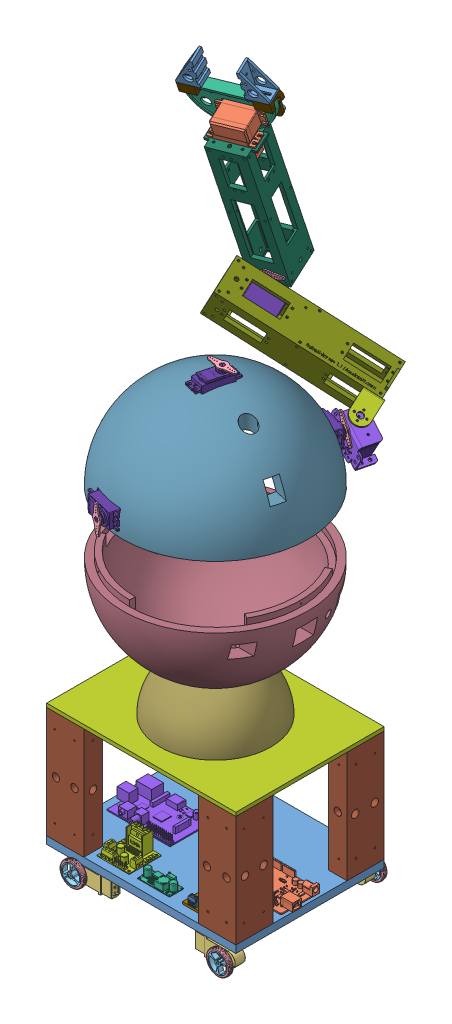
SolidWorks assembly Capitulo05b, configuration Default. Lengths in mm.
Overall size (318.26 870.37 456.14).
92 component instances, 43 part files, 77 mates.
Components (placement in the parent):
- BaseRodas-1: BaseRodas [Valor predeterminado] at (85.4958 105.7561 216.0087) size (255 10 200)
- ArduinoMega-1: ArduinoMega [Default] at (157.8742 117.4071 223.7908) x (1 0 0) z (0 -1 0) size (107.95 53.42 12.95)
- Pololu Motor-1: Pololu Motor [Default] at (-2.4413 93.3561 314.8723) size (58.5 24.8 23.8)
- Pololu Motor-2: Pololu Motor [Default] at (202.1148 93.3561 316.3087) x (-1 0 0) z (0 0 1) size (58.5 24.8 23.8)
- Pololu Motor-3: Pololu Motor [Default] at (-25.2153 93.3561 115.7087) x (1 0 0) z (0 0 -1) size (58.5 24.8 23.8)
- Pololu Motor-4: Pololu Motor [Default] at (191.7418 93.3561 115.7087) x (-1 0 0) z (0 0 -1) size (58.5 24.8 23.8)
- Pololu-Wheel-32x7mm-1: Pololu-Wheel-32x7mm [По умолчанию] at (199.6861 93.3761 327.4608) x (0 0 -1) z (-1 0 0) size (8.53 32.01 32.01)
  - Pololu-Wheel-32x7mm-tire-2: Pololu-Wheel-32x7mm-tire [По умолчанию] at (0.25 0 0) size (6 32.01 32.01)
  - Pololu-Wheel-32x7mm-rim-1: Pololu-Wheel-32x7mm-rim [По умолчанию] x (0 0 -1) z (0 -1 0) size (28.4 8.53 28.4)
- Pololu-Wheel-32x7mm-2: Pololu-Wheel-32x7mm [По умолчанию] at (-2.4611 93.3361 316.0712) x (0 0 1) z (-1 0 0) size (8.53 32.01 32.01)
  - Pololu-Wheel-32x7mm-tire-2: Pololu-Wheel-32x7mm-tire [По умолчанию] at (0.25 0 0) size (6 32.01 32.01)
  - Pololu-Wheel-32x7mm-rim-1: Pololu-Wheel-32x7mm-rim [По умолчанию] x (0 0 -1) z (0 -1 0) size (28.4 8.53 28.4)
- Pololu-Wheel-32x7mm-3: Pololu-Wheel-32x7mm [По умолчанию] at (-25.2515 93.3761 107.2669) x (0 0 1) z (1 0 0) size (8.53 32.01 32.01)
  - Pololu-Wheel-32x7mm-tire-2: Pololu-Wheel-32x7mm-tire [По умолчанию] at (0.25 0 0) size (6 32.01 32.01)
  - Pololu-Wheel-32x7mm-rim-1: Pololu-Wheel-32x7mm-rim [По умолчанию] x (0 0 -1) z (0 -1 0) size (28.4 8.53 28.4)
- Pololu-Wheel-32x7mm-4: Pololu-Wheel-32x7mm [По умолчанию] at (191.7625 93.3361 105.8111) x (0 0 1) z (-1 0 0) size (8.53 32.01 32.01)
  - Pololu-Wheel-32x7mm-tire-2: Pololu-Wheel-32x7mm-tire [По умолчанию] at (0.25 0 0) size (6 32.01 32.01)
  - Pololu-Wheel-32x7mm-rim-1: Pololu-Wheel-32x7mm-rim [По умолчанию] x (0 0 -1) z (0 -1 0) size (28.4 8.53 28.4)
- stepdown voltage converter-1: stepdown voltage converter [Default] at (91.0071 115.7561 295.2838) x (1 0 0) z (0 1 0) size (42.85 19.13 11.5)
- L298N-1: L298N [Predeterminado] at (58.7836 115.7561 262.3157) size (43.3 25 43.3)
- raspberry pi-1: raspberry pi [Default] at (11.5976 115.7561 217.2219) x (1 0 0) z (0 1 0) size (90.8 63.5 15.5)
- Sensor Tensão-1: Sensor Tensão [Default] at (126.3749 100.0519 260.3458) size (25 13.5 35)
  - Sensor Corrente-1: Sensor Corrente [Default] at (2.9759 15.7042 43.8137) size (25 3 35)
  - Borne-1: Borne [Default] at (14.7854 18.7042 40.29) size (11.16 13.5 7.5)
- Prolongador-1: Prolongador [Default] at (-42.0042 115.7561 316.0087) size (50 150 50)
- Prolongador-2: Prolongador [Default] at (212.9958 115.7561 316.0087) x (0 0 -1) z (1 0 0) size (50 150 50)
- Prolongador-3: Prolongador [Default] at (212.9958 115.7561 116.0087) x (-1 0 0) z (0 0 -1) size (50 150 50)
- Prolongador-4: Prolongador [Default] at (-42.0042 115.7561 116.0087) x (0 0 1) z (-1 0 0) size (50 150 50)
- BasePeqInf-1: BasePeqInf [Valor predeterminado] at (85.4958 270.7561 216.0087) x (1 0 0) z (0 -1 0) size (149.62 150 66.73)
- BaseGrandeInf-2: BaseGrandeInf [Valor predeterminado] at (85.4958 454.6169 216.0087) x (0 0 1) z (0 1 0) size (250 250 133)
- BaseGrandeSup-1: BaseGrandeSup [Valor predeterminado] at (85.4958 538.3008 216.0087) x (0.972129 0 0.234447) z (0 -1 0) size (250 250 133)
- montagem  braço-1: montagem  braço [Default] at (-170.3433 856.3022 -7.132) x (0.003785 -0.950278 -0.311379) z (0.26972 -0.298871 0.915384) size (413.65 211.91 175.32)
  - BRACO_BASE-1: BRACO_BASE [Valor predeterminado] at (14.84 86.0383 96.2487) size (190 59 48)
  - BRACO_EXTENSAO-1: BRACO_EXTENSAO [Valor predeterminado] at (256.4141 254.3736 159.7487) x (-0.539485 -0.841995 0) z (0 0 1) size (190 59 48)
  - HS-475HB_001-1: HS-475HB_001 [Default] at (198.2651 118.9459 184.2487) x (0.539485 0.841995 0) z (-0.841995 0.539485 0) size (53 41.6 19.8)
  - 1499-1: 1499 [Predeterminado] at (5.84 129.3383 110.6487) x (0 -1 0) z (0 0 -1) size (105.2 141.1 49.07)
    - base pinza-1: base pinza [Predeterminado] at (50.3318 68.1 -0.4295) x (0.999944 0 -0.01061) z (0.01061 0 0.999944) size (20 40.4 23.6)
    - base pinza-2: base pinza [Predeterminado] at (-33.0716 68 0.4555) x (0.999944 0 -0.01061) z (0.01061 0 0.999944) size (20 40.4 23.6)
    - pinza-1: pinza [Predeterminado] at (33.0328 68.1 -0.246) x (0.999944 0 -0.01061) z (0.01061 0 0.999944) size (27.3 38 20.4)
    - pinza-2: pinza [Predeterminado] at (-15.9901 68 -20.2269) x (-0.999944 0 0.01061) z (-0.01061 0 -0.999944) size (27.3 38 20.4)
    - Servo4.3kilos_TR205-1: Servo4.3kilos_TR205 [Predeterminado] at (19.1276 46.95 -7.2488) x (-0.999944 0 0.01061) z (0 1 0) size (54.6 44.5 19.6)
    - corona 1 servo 4.3 Kg.-1: corona 1 servo 4.3 Kg. [Predeterminado] at (9.8 11.5 -9.8) x (0.01061 0 0.999944) z (-0.999944 0 0.01061) size (20.9 6 20.9)
    - corona 1 servo 3.4 Kg.-1: corona 1 servo 3.4 Kg. [Predeterminado] at (9.4427 37.15 3.6545) x (-0.271943 0.962309 0.002886) z (-0.962255 -0.271958 0.01021) size (13.7 3.8 38.7)
    - brazo curvo-1: brazo curvo [Predeterminado] at (43.5627 53.1085 5.8926) x (0.941753 -0.336157 -0.009993) z (0.336138 0.941806 -0.003567) size (35 2.6 13)
    - brazo curvo-2: brazo curvo [Predeterminado] at (-19.7488 49.5562 6.5644) x (0.999941 0.002524 -0.01061) z (-0.002524 0.999997 0.000027) size (35 2.6 13)
    - Servo4.3kilos_TR205-2: Servo4.3kilos_TR205 [Predeterminado] at origin size (54.6 44.5 19.6)
    - riel-2: riel [Predeterminado] at (9.8 64 -9.8) x (0.999944 0 -0.01061) z (0.01061 0 0.999944) size (104 52.5 21.9)
  - corona 1 servo 3.4 Kg.-1: corona 1 servo 3.4 Kg. [Predeterminado] at (193.14 110.9469 142.2487) x (0.9993 0.03741 0) z (0.03741 -0.9993 0) size (13.7 3.8 38.7)
  - U Bracket1-1: U Bracket1 [Default] at (273.3664 232.823 205.7487) x (0.841995 -0.539485 0) z (-0.539485 -0.841995 0) size (56 42 24)
  - Multi Purpose Bracket-1: Multi Purpose Bracket [Default] at (253.4429 244.7315 253.2461) x (-0.445957 -0.696023 -0.562737) z (0.841995 -0.539485 0) size (58 27 37.5)
  - Horn-1: Horn [Default] at (295.2583 218.7963 235.7487) x (0.539485 0.841995 0) z (0 0 -1) size (24 5 24)
  - HS-475HB_001-2: HS-475HB_001 [Default] at (263.5417 248.4446 241.0947) x (0.445957 0.696023 0.562737) z (0.303588 0.473822 -0.826636) size (53 41.6 19.8)
- HS-475HB_001-2: HS-475HB_001 [Default] at (108.4917 558.9008 120.2306) x (-0.972129 0 -0.234447) z (0 -1 0) size (53 41.6 19.8)
- HS-475HB_001-3: HS-475HB_001 [Default] at (64.8331 558.2008 312.3495) x (-0.972129 0 -0.234447) z (0 1 0) size (53 41.6 19.8)
- corona 1 servo 3.4 Kg.-1: corona 1 servo 3.4 Kg. [Predeterminado] at (127.5737 558.9008 81.6284) x (-0.844064 -0.496104 -0.203562) z (-0.482277 0.868263 -0.11631) size (13.7 3.8 38.7)
- LCD-1: LCD [Default] at (-9.8148 566.4008 192.3541) x (-0.234447 0 0.972129) z (0 -1 0) size (79.73 22.63 31.99)
  - 16pin_header__-1: 16pin_header__ [Default] at (-32 0 -15.5) x (0 0 1) z (1 0 0) size (2.54 11.5 40.64)
  - lcd window-1: lcd window [Default] at (0 9 1.5) size (71.3 11.8 27.44)
  - backlight-1: backlight [Default] at (0 1.7 1.5) x (-1 0 0) z (0 0 -1) size (74.38 2.98 18)
  - conductor-1: conductor [Default] at (0 1.7 12.6) size (69.7 5.5 3)
  - conductor-2: conductor [Default] at (0 1.7 -9.6) size (69.7 5.5 3)
  - liquid crystal grabcad i2s-1: liquid crystal grabcad i2s [Default] at (0 7.9 1.5) size (68.5 2.2 25)
  - smt_resistor222-1: smt_resistor222 [Default] at (-32.75 0 -5.25) x (0 0 1) z (1 0 0) size (1.8 0.6 4)
  - smt_resistor222-2: smt_resistor222 [Default] at (-32.75 0 -2.75) x (0 0 1) z (1 0 0) size (1.8 0.6 4)
  - smt_resistor222-3: smt_resistor222 [Default] at (-32.75 0 -0.25) x (0 0 1) z (1 0 0) size (1.8 0.6 4)
  - smt_resistor222-4: smt_resistor222 [Default] at (-32.75 0 2.25) x (0 0 1) z (1 0 0) size (1.8 0.6 4)
  - smt_resistor222-5: smt_resistor222 [Default] at (-32.75 0 4.75) x (0 0 1) z (1 0 0) size (1.8 0.6 4)
  - smt_resistor222-6: smt_resistor222 [Default] at (-32.75 0 7.25) x (0 0 1) z (1 0 0) size (1.8 0.6 4)
  - smt_resistor101-1: smt_resistor101 [Default] at (30.25 0 6.1) x (0 0 -1) z (-1 0 0) size (1.8 0.6 5.2)
  - smt_resistor101-2: smt_resistor101 [Default] at (30.25 0 2.85) x (0 0 -1) z (-1 0 0) size (1.8 0.6 5.2)
  - i2c board-1: i2c board [Default] at (6.1 -5 -15.5) x (-1 0 0) z (0 0 1) size (54.1 8.62 19.35)
    - i2C board-1: i2C board [Default] at origin size (40.64 1.8 19.35)
    - jumper__-1: jumper__ [Default] at (-0.2258 6.825 6.38) x (0 0 -1) z (0 1 0) size (5 6 2)
    - pcf8574p-1: pcf8574p [Default] at (17.78 1.6 7.62) size (11.9 2.51 10.2)
    - bent header-1: bent header [Default] at (38.1 1.7 5.08) x (0 0 1) z (-1 0 0) size (2.54 8 9.27)
    - led-1: led [Default] at (2.54 1.6 10.16) x (0 0 -1) z (1 0 0) size (4 0.86 1.35)
    - ssot3-1: ssot3 [Default] at (4.1275 1.6 5.08) size (3 1.13 3.09)
    - trimpot 3662-1: trimpot 3662 [Default] at (29.21 1.6 7.62) size (6.6 6.67 6.99)
    - smt_resistor222-2: smt_resistor222 [Default] at (10.16 1.6 10.16) size (1.8 0.6 4)
    - smt_resistor222-3: smt_resistor222 [Default] at (7.62 1.6 10.16) size (1.8 0.6 4)
    - smt_resistor222-4: smt_resistor222 [Default] at (5.08 1.6 10.16) size (1.8 0.6 4)
    - smt_resistor222-5: smt_resistor222 [Default] at (7.62 1.6 5.08) size (1.8 0.6 4)
    - bent header-3: bent header [Default] at (0 1.7 5.08) x (0 0 -1) z (1 0 0) size (2.54 8 9.27)
    - bent header-4: bent header [Default] at (0 1.7 7.62) x (0 0 -1) z (1 0 0) size (2.54 8 9.27)
    - bent header-5: bent header [Default] at (38.1 1.7 7.62) x (0 0 1) z (-1 0 0) size (2.54 8 9.27)
    - bent header-6: bent header [Default] at (38.1 1.7 10.16) x (0 0 1) z (-1 0 0) size (2.54 8 9.27)
    - bent header-7: bent header [Default] at (38.1 1.7 12.7) x (0 0 1) z (-1 0 0) size (2.54 8 9.27)
    - smt_cap-2: smt_cap [Default] at (10.16 1.6 5.08) x (-1 0 0) z (0 0 -1) size (1.8 1 4)
- HS-475HB_001-4: HS-475HB_001 [Default] at (87.0418 636.8008 219.6219) x (-0.234447 0 0.972129) z (-0.972129 0 -0.234447) size (53 41.6 19.8)
- corona 1 servo 3.4 Kg.-2: corona 1 servo 3.4 Kg. [Predeterminado] at (64.2216 558.2008 355.4062) x (-0.96849 -0.086447 -0.23357) z (0.084038 -0.996256 0.020267) size (13.7 3.8 38.7)
- corona 1 servo 3.4 Kg.-3: corona 1 servo 3.4 Kg. [Predeterminado] at (89.2691 678.8008 210.3867) x (0.013394 0 -0.99991) z (-0.99991 0 -0.013394) size (13.7 3.8 38.7)
- BaseReta-2: BaseReta [Default] at (-42.0042 270.7561 116.0087) x (1 0 0) z (0 -1 0) size (255 200 5)
Mates (geometry in assembly coordinates):
- Coincident2: coincident anti-aligned: plane of BaseRodas-1 through (212.9958 115.7561 116.0087) normal (0 1 0); plane of ArduinoMega-1 through (208.6742 115.7561 197.0827) normal (0 -1 0)
- Coincident4: coincident anti-aligned: plane of BaseRodas-1 through (212.9958 105.7561 116.0087) normal (0 -1 0); plane of Pololu Motor-1 through (29.0587 105.7561 300.7723) normal (0 1 0)
- Coincident6: coincident anti-aligned: plane of BaseRodas-1 through (212.9958 105.7561 116.0087) normal (0 -1 0); plane of Pololu Motor-4 through (160.2418 105.7561 129.8087) normal (0 1 0)
- Coincident10: coincident aligned: plane of BaseRodas-1 through (-42.0042 115.7561 116.0087) normal (0 0 -1); plane of Pololu Motor-4 through (191.7418 93.3561 116.0087) normal (0 0 -1)
- Coincident11: coincident: plane of BaseRodas-1 through (212.9958 105.7561 116.0087) normal (0 -1 0); line of Pololu Motor-3 through (3.4347 105.7561 116.1587) axis (0 0 1)
- Coincident13: coincident aligned: plane of BaseRodas-1 through (-42.0042 115.7561 116.0087) normal (0 0 -1); plane of Pololu Motor-3 through (-25.2153 93.3561 116.0087) normal (0 0 -1)
- Parallel2: parallel aligned: plane of BaseRodas-1 through (212.9958 105.7561 116.0087) normal (0 -1 0); plane of Pololu Motor-3 through (6.2847 80.9561 129.8087) normal (0 -1 0)
- Parallel3: parallel aligned: plane of BaseRodas-1 through (-42.0042 115.7561 316.0087) normal (0 0 1); plane of Pololu Motor-2 through (202.1148 93.3561 316.0087) normal (0 0 1)
- Parallel4: parallel aligned: plane of BaseRodas-1 through (212.9958 105.7561 116.0087) normal (0 -1 0); plane of Pololu Motor-2 through (170.6148 80.9561 302.2087) normal (0 -1 0)
- Coincident17: coincident anti-aligned: plane of BaseRodas-1 through (212.9958 105.7561 116.0087) normal (0 -1 0); plane of Pololu Motor-2 through (170.6148 105.7561 302.2087) normal (0 1 0)
- Coincident18: coincident aligned: plane of BaseRodas-1 through (-42.0042 115.7561 316.0087) normal (0 0 1); plane of Pololu Motor-2 through (202.1148 93.3561 316.0087) normal (0 0 1)
- Coincident24: coincident anti-aligned: plane of Pololu Motor-2 through (203.2503 92.3761 316.0087) normal (0 -1 0); plane of Pololu-Wheel-32x7mm-1/Pololu-Wheel-32x7mm-rim-1 through (198.568 92.3761 327.4608) normal (0 1 0)
- Parallel11: parallel aligned: cylinder of Pololu Motor-2 through (202.1148 93.3561 316.0087) axis (0 0 1) radius 1.5; cylinder of Pololu-Wheel-32x7mm-1/Pololu-Wheel-32x7mm-rim-1 through (199.6861 93.3761 320.9608) axis (0 0 1) radius 1.5
- Parallel15: parallel anti-aligned: plane of Pololu Motor-1 through (-2.4413 93.3561 324.5723) normal (0 0 1); plane of Pololu-Wheel-32x7mm-2/Pololu-Wheel-32x7mm-rim-1 through (-2.4611 93.3361 316.0712) normal (0 0 -1)
- Coincident27: coincident anti-aligned: plane of Pololu Motor-1 through (-3.5768 94.3361 314.5723) normal (0 1 0); plane of Pololu-Wheel-32x7mm-2/Pololu-Wheel-32x7mm-rim-1 through (-3.5792 94.3361 316.0712) normal (0 -1 0)
- Parallel21: parallel aligned: plane of Pololu Motor-3 through (-25.2153 93.3561 106.0087) normal (0 0 -1); plane of Pololu-Wheel-32x7mm-3/Pololu-Wheel-32x7mm-rim-1 through (-25.2515 93.3761 107.2669) normal (0 0 -1)
- Coincident36: coincident anti-aligned: plane of Pololu Motor-3 through (-26.3508 92.3761 116.0087) normal (0 -1 0); plane of Pololu-Wheel-32x7mm-3/Pololu-Wheel-32x7mm-rim-1 through (-24.1334 92.3761 107.2669) normal (0 1 0)
- Parallel22: parallel aligned: plane of Pololu Motor-4 through (191.7418 93.3561 106.0087) normal (0 0 -1); plane of Pololu-Wheel-32x7mm-4/Pololu-Wheel-32x7mm-rim-1 through (191.7625 93.3361 105.8111) normal (0 0 -1)
- Coincident38: coincident anti-aligned: plane of Pololu Motor-4 through (192.8774 94.3361 116.0087) normal (0 1 0); plane of Pololu-Wheel-32x7mm-4/Pololu-Wheel-32x7mm-rim-1 through (190.6444 94.3361 105.8111) normal (0 -1 0)
- Coincident39: coincident anti-aligned: plane of BaseRodas-1 through (212.9958 115.7561 116.0087) normal (0 1 0); plane of stepdown voltage converter-1 through (91.0071 115.7561 295.2838) normal (0 -1 0)
- Coincident40: coincident anti-aligned: plane of BaseRodas-1 through (212.9958 115.7561 116.0087) normal (0 1 0); plane of L298N-1 through (-10.6379 115.7561 283.9657) normal (0 -1 0)
- Coincident42: coincident anti-aligned: plane of BaseRodas-1 through (212.9958 115.7561 116.0087) normal (0 1 0); plane of raspberry pi-1 through (11.5976 115.7561 217.2219) normal (0 -1 0)
- Coincident43: coincident anti-aligned: plane of BaseRodas-1 through (212.9958 115.7561 116.0087) normal (0 1 0); plane of Sensor Tensão-1/Sensor Corrente-1 through (129.3508 115.7561 304.1595) normal (0 -1 0)
- Coincident45: coincident anti-aligned: plane of BaseRodas-1 through (212.9958 115.7561 116.0087) normal (0 1 0); plane of Prolongador-1 through (-42.0042 115.7561 316.0087) normal (0 -1 0)
- Coincident46: coincident aligned: plane of BaseRodas-1 through (-42.0042 115.7561 316.0087) normal (0 0 1); plane of Prolongador-1 through (-42.0042 265.7561 316.0087) normal (0 0 1)
- Parallel24: parallel aligned: plane of BaseRodas-1 through (-42.0042 115.7561 316.0087) normal (0 0 1); plane of Prolongador-2 through (212.9958 265.7561 316.0087) normal (0 0 1)
- Parallel25: parallel aligned: plane of BaseRodas-1 through (212.9958 115.7561 316.0087) normal (1 0 0); plane of Prolongador-2 through (212.9958 265.7561 316.0087) normal (1 0 0)
- Coincident49: coincident anti-aligned: plane of BaseRodas-1 through (212.9958 115.7561 116.0087) normal (0 1 0); plane of Prolongador-2 through (212.9958 115.7561 316.0087) normal (0 -1 0)
- Parallel27: parallel aligned: plane of BaseRodas-1 through (212.9958 115.7561 316.0087) normal (1 0 0); plane of Prolongador-3 through (212.9958 265.7561 116.0087) normal (1 0 0)
- Parallel28: parallel aligned: plane of BaseRodas-1 through (-42.0042 115.7561 116.0087) normal (0 0 -1); plane of Prolongador-3 through (212.9958 265.7561 116.0087) normal (0 0 -1)
- Coincident55: coincident: point of BaseRodas-1; moEndPointRef_w of Prolongador-3
- Parallel29: parallel aligned: plane of BaseRodas-1 through (-42.0042 115.7561 116.0087) normal (0 0 -1); plane of Prolongador-4 through (-42.0042 265.7561 116.0087) normal (0 0 -1)
- Parallel30: parallel aligned: plane of BaseRodas-1 through (-42.0042 115.7561 316.0087) normal (-1 0 0); plane of Prolongador-4 through (-42.0042 265.7561 116.0087) normal (-1 0 0)
- Coincident58: coincident: point of BaseRodas-1; point of Prolongador-4
- Concentric5: concentric anti-aligned: circle of BaseGrandeInf-2; circle of BaseGrandeSup-1
- Parallel35: parallel anti-aligned: plane of BaseGrandeSup-1 through (95.8452 568.8008 89.9209) normal (0.972129 0 0.234447); plane of HS-475HB_001-2 through (98.0725 568.8008 80.6857) normal (-0.972129 0 -0.234447)
- Parallel36: parallel anti-aligned: plane of BaseGrandeSup-1 through (136.0914 568.8008 99.627) normal (0 -1 0); plane of HS-475HB_001-2 through (135.7911 568.8008 89.7822) normal (0 1 0)
- Parallel37: parallel anti-aligned: plane of BaseGrandeSup-1 through (136.0914 548.3008 99.627) normal (-0.972129 0 -0.234447); plane of HS-475HB_001-2 through (135.7911 568.8008 89.7822) normal (0.972129 0 0.234447)
- Tangent1: tangent anti-aligned: sphere of BaseGrandeSup-1; plane of HS-475HB_001-2 through (140.4659 549.6008 100.682) normal (-0.234447 0 0.972129)
- Coincident73: coincident anti-aligned: circle of BaseGrandeSup-1; plane of HS-475HB_001-2 through (98.0725 568.8008 80.6857) normal (-0.972129 0 -0.234447)
- Coincident74: coincident anti-aligned: circle of BaseGrandeSup-1; plane of HS-475HB_001-2 through (135.7911 568.8008 89.7822) normal (0 1 0)
- Parallel38: parallel anti-aligned: plane of BaseGrandeSup-1 through (95.8452 548.3008 89.9209) normal (0 1 0); plane of HS-475HB_001-3 through (75.2523 548.3008 351.8944) normal (0 -1 0)
- Coincident77: coincident anti-aligned: plane of BaseGrandeSup-1 through (136.0914 548.3008 99.627) normal (-0.972129 0 -0.234447); plane of HS-475HB_001-3 through (75.2523 548.3008 351.8944) normal (0.972129 0 0.234447)
- Coincident78: coincident anti-aligned: plane of BaseGrandeSup-1 through (95.8452 548.3008 89.9209) normal (0 1 0); plane of HS-475HB_001-3 through (75.2523 548.3008 351.8944) normal (0 -1 0)
- Tangent2: tangent anti-aligned: sphere of BaseGrandeSup-1; plane of HS-475HB_001-3 through (32.8589 567.5008 331.8981) normal (0.234447 0 -0.972129)
- Concentric6: concentric aligned: cylinder of HS-475HB_001-2 through (139.1394 558.9008 33.6716) axis (-0.234447 0 0.972129) radius 2.875; cylinder of corona 1 servo 3.4 Kg.-1 through (127.2689 558.9008 82.8922) axis (-0.234447 0 0.972129) radius 2.7
- Coincident81: coincident anti-aligned: circle of HS-475HB_001-2; plane of corona 1 servo 3.4 Kg.-1 through (126.6828 558.9008 85.3225) normal (-0.234447 0 0.972129)
- Coincident84: coincident anti-aligned: plane of montagem  braço-1/Multi Purpose Bracket-1 through (117.6956 572.0624 79.2461) normal (-0.234447 0 0.972129); plane of corona 1 servo 3.4 Kg.-1 through (135.6518 544.3574 83.5766) normal (0.234447 0 -0.972129)
- Concentric7: concentric anti-aligned: circle of montagem  braço-1/Multi Purpose Bracket-1; circle of corona 1 servo 3.4 Kg.-1
- Parallel45: parallel anti-aligned: plane of BaseGrandeSup-1 through (-27.8146 553.9008 152.6783) normal (-0.234447 0 0.972129); plane of LCD-1/lcd window-1 through (-8.2617 573.5008 156.0566) normal (0.234447 0 -0.972129)
- Parallel46: parallel anti-aligned: plane of BaseGrandeSup-1 through (-44.2259 553.9008 220.7273) normal (0 1 0); plane of LCD-1/lcd window-1 through (-18.564 551.5008 190.2441) normal (0 -1 0)
- Coincident93: coincident anti-aligned: plane of BaseGrandeSup-1 through (-44.2259 578.3008 220.7273) normal (0 -1 0); plane of LCD-1/lcd window-1 through (-18.564 578.3008 190.2441) normal (0 1 0)
- Coincident94: coincident anti-aligned: plane of BaseGrandeSup-1 through (-44.2259 553.9008 220.7273) normal (0.234447 0 -0.972129); plane of LCD-1/lcd window-1 through (-24.9778 556.3008 225.3694) normal (-0.234447 0 0.972129)
- Tangent3: tangent aligned: sphere of BaseGrandeSup-1; plane of LCD-1/lcd window-1 through (-19.3417 564.9008 190.0565) normal (-0.972129 0 -0.234447)
- Parallel47: parallel anti-aligned: plane of BaseGrandeSup-1 through (101.2142 663.3008 203.0836) normal (-0.972129 0 -0.234447); plane of HS-475HB_001-4 through (101.2142 672.8008 203.0836) normal (0.972129 0 0.234447)
- Coincident97: coincident anti-aligned: plane of BaseGrandeSup-1 through (80.7995 663.3008 198.1602) normal (-0.234447 0 0.972129); plane of HS-475HB_001-4 through (101.2142 672.8008 203.0836) normal (0.234447 0 -0.972129)
- Coincident98: coincident anti-aligned: plane of BaseGrandeSup-1 through (101.2142 663.3008 203.0836) normal (-0.972129 0 -0.234447); plane of HS-475HB_001-4 through (101.2142 672.8008 203.0836) normal (0.972129 0 0.234447)
- Tangent4: tangent anti-aligned: sphere of BaseGrandeSup-1; plane of HS-475HB_001-4 through (71.7882 663.3008 243.2029) normal (0 -1 0)
- Concentric8: concentric aligned: cylinder of HS-475HB_001-3 through (52.6559 558.2008 403.363) axis (0.234447 0 -0.972129) radius 2.875; cylinder of corona 1 servo 3.4 Kg.-2 through (64.5263 558.2008 354.1424) axis (0.234447 0 -0.972129) radius 2.7
- Coincident99: coincident anti-aligned: plane of HS-475HB_001-3 through (65.1125 558.2008 351.7121) normal (-0.234447 0 0.972129); plane of corona 1 servo 3.4 Kg.-2 through (65.1125 558.2008 351.7121) normal (0.234447 0 -0.972129)
- Concentric9: concentric aligned: cylinder of HS-475HB_001-4 through (89.2691 728.1326 210.3867) axis (0 -1 0) radius 2.875; cylinder of corona 1 servo 3.4 Kg.-3 through (89.2691 677.5008 210.3867) axis (0 -1 0) radius 2.7
- Coincident100: coincident anti-aligned: plane of HS-475HB_001-4 through (89.2691 675.0008 210.3867) normal (0 1 0); plane of corona 1 servo 3.4 Kg.-3 through (89.2691 675.0008 210.3867) normal (0 -1 0)
- Parallel48: parallel anti-aligned: line of Prolongador-4 through (-42.0042 265.7561 116.0087) axis (0 0 1); line of BaseReta-2 through (-42.0042 270.7561 316.0087) axis (0 0 -1)
- Parallel49: parallel anti-aligned: line of Prolongador-4 through (7.9958 265.7561 116.0087) axis (-1 0 0); line of BaseReta-2 through (-42.0042 270.7561 116.0087) axis (1 0 0)
- Coincident103: coincident: point of Prolongador-1; point of BaseReta-2
- Concentric10: concentric aligned: circle of BasePeqInf-1; circle of BaseReta-2
- Coincident105: coincident anti-aligned: line of Prolongador-2 through (212.9958 265.7561 316.0087) axis (0 0 -1); line of BaseReta-2 through (212.9958 265.7561 116.0087) axis (0 0 1)
- Coincident106: coincident aligned: line of BaseRodas-1 through (212.9958 115.7561 316.0087) axis (0 0 -1); line of Prolongador-2 through (212.9958 115.7561 316.0087) axis (0 0 -1)
- Concentric11: concentric aligned: circle of BasePeqInf-1; circle of BaseReta-2
- Coincident109: coincident aligned: line of BaseRodas-1 through (-42.0042 115.7561 316.0087) axis (1 0 0); line of Prolongador-2 through (162.9958 115.7561 316.0087) axis (1 0 0)
- Concentric13: concentric anti-aligned: circle of BasePeqInf-1; circle of BaseReta-2
- Concentric14: concentric anti-aligned: circle of BasePeqInf-1; circle of BaseReta-2
- Coincident112: coincident anti-aligned: plane of BasePeqInf-1 through (85.4958 270.7561 216.0087) normal (0 -1 0); plane of BaseReta-2 through (-42.0042 270.7561 116.0087) normal (0 1 0)
- Concentric15: concentric anti-aligned: circle of BasePeqInf-1; circle of BaseGrandeInf-2
- Concentric16: concentric aligned: circle of BasePeqInf-1; circle of BaseGrandeInf-2
- Concentric17: concentric aligned: circle of BasePeqInf-1; circle of BaseGrandeInf-2
- Coincident116: coincident anti-aligned: plane of BasePeqInf-1 through (50.4958 337.4886 266.0087) normal (0 1 0); plane of BaseGrandeInf-2 through (-39.5042 337.4886 284.3117) normal (0 -1 0)
